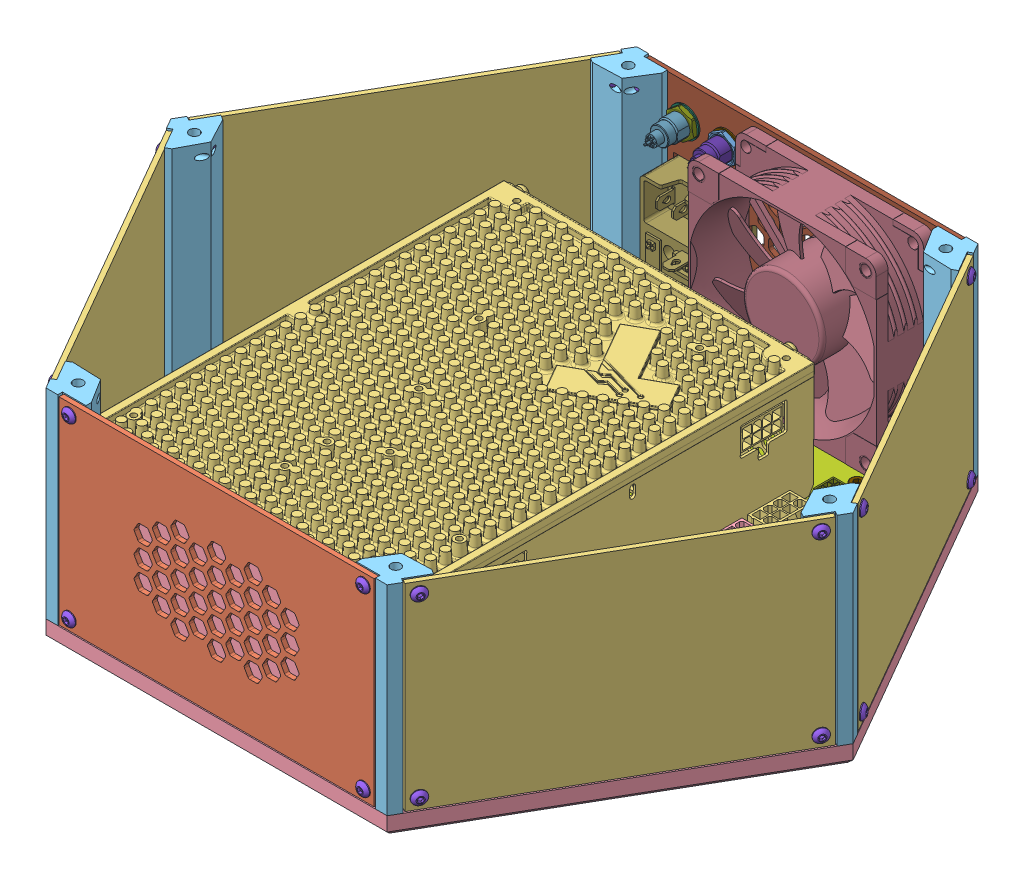
SolidWorks assembly base_assembly, configuration Default. Lengths in mm. (continued)
Components (placement in the parent): (continued)
- zaphod-controller-1: zaphod-controller [Default] at (56 14 107.9) x (0 0 -1) z (0 1 0) size (199.92 69.34 18.57) (continued)
  - SOT95P240X110-3L16-18: SOT95P240X110-3L16 [Default] at (114 -66.9 1.65) size (2.91 3.01 1.23) (continued)
    - COMPOUND_6-1: COMPOUND_6 [Default] at origin size (2.91 3.01 1.23)
  - SOT95P240X110-3L16-19: SOT95P240X110-3L16 [Default] at (114 -61.2 1.65) size (2.91 3.01 1.23)
    - COMPOUND_6-1: COMPOUND_6 [Default] at origin size (2.91 3.01 1.23)
  - SOT95P240X110-3L16-20: SOT95P240X110-3L16 [Default] at (141.5 -23.1 1.65) x (0 -1 0) z (0 0 1) size (2.91 3.01 1.23)
    - COMPOUND_6-1: COMPOUND_6 [Default] at origin size (2.91 3.01 1.23)
  - SOT95P240X110-3L16-21: SOT95P240X110-3L16 [Default] at (122.4 -45.4 1.65) x (-1 0 0) z (0 0 1) size (2.91 3.01 1.23)
    - COMPOUND_6-1: COMPOUND_6 [Default] at origin size (2.91 3.01 1.23)
  - RESC1608X50-9: RESC1608X50 [Default] at (169.2907 -2.1731 -0.05) x (1 0 0) z (0 0 -1) size (1.6 0.8 0.5)
    - COMPOUND_5-1: COMPOUND_5 [Default] at origin size (1.6 0.8 0.5)
  - RESC1608X50-10: RESC1608X50 [Default] at (169.2907 -4.1731 -0.05) x (-1 0 0) z (0 0 -1) size (1.6 0.8 0.5)
    - COMPOUND_5-1: COMPOUND_5 [Default] at origin size (1.6 0.8 0.5)
  - RESC1608X50-11: RESC1608X50 [Default] at (169.2907 -6.1731 -0.05) x (1 0 0) z (0 0 -1) size (1.6 0.8 0.5)
    - COMPOUND_5-1: COMPOUND_5 [Default] at origin size (1.6 0.8 0.5)
  - RESC1608X50-12: RESC1608X50 [Default] at (103 -51 1.65) x (0 -1 0) z (0 0 1) size (1.6 0.8 0.5)
    - COMPOUND_5-1: COMPOUND_5 [Default] at origin size (1.6 0.8 0.5)
  - RESC1608X50-13: RESC1608X50 [Default] at (32.7 -21 1.65) x (-1 0 0) z (0 0 1) size (1.6 0.8 0.5)
    - COMPOUND_5-1: COMPOUND_5 [Default] at origin size (1.6 0.8 0.5)
  - RESC1608X50-14: RESC1608X50 [Default] at (29.2 -19.75 1.65) size (1.6 0.8 0.5)
    - COMPOUND_5-1: COMPOUND_5 [Default] at origin size (1.6 0.8 0.5)
  - RESC1608X50-15: RESC1608X50 [Default] at (96.275 -42.75 1.65) x (-1 0 0) z (0 0 1) size (1.6 0.8 0.5)
    - COMPOUND_5-1: COMPOUND_5 [Default] at origin size (1.6 0.8 0.5)
  - RESC1608X50-16: RESC1608X50 [Default] at (106.5 -51 1.65) x (0 1 0) z (0 0 1) size (1.6 0.8 0.5)
    - COMPOUND_5-1: COMPOUND_5 [Default] at origin size (1.6 0.8 0.5)
  - RESC1608X50-17: RESC1608X50 [Default] at (106.5 -47.5 1.65) x (0 1 0) z (0 0 1) size (1.6 0.8 0.5)
    - COMPOUND_5-1: COMPOUND_5 [Default] at origin size (1.6 0.8 0.5)
  - RESC1608X50-18: RESC1608X50 [Default] at (32.7 -18 1.65) x (-1 0 0) z (0 0 1) size (1.6 0.8 0.5)
    - COMPOUND_5-1: COMPOUND_5 [Default] at origin size (1.6 0.8 0.5)
  - RESC1608X50-19: RESC1608X50 [Default] at (29.2 -18 1.65) x (-1 0 0) z (0 0 1) size (1.6 0.8 0.5)
    - COMPOUND_5-1: COMPOUND_5 [Default] at origin size (1.6 0.8 0.5)
  - RESC1608X50-20: RESC1608X50 [Default] at (32.7 -27 1.65) x (-1 0 0) z (0 0 1) size (1.6 0.8 0.5)
    - COMPOUND_5-1: COMPOUND_5 [Default] at origin size (1.6 0.8 0.5)
  - RESC1608X50-21: RESC1608X50 [Default] at (29.45 -28.75 1.65) x (-1 0 0) z (0 0 1) size (1.6 0.8 0.5)
    - COMPOUND_5-1: COMPOUND_5 [Default] at origin size (1.6 0.8 0.5)
  - RESC1608X50-22: RESC1608X50 [Default] at (32.7 -28.75 1.65) x (-1 0 0) z (0 0 1) size (1.6 0.8 0.5)
    - COMPOUND_5-1: COMPOUND_5 [Default] at origin size (1.6 0.8 0.5)
  - RESC1608X50-23: RESC1608X50 [Default] at (41.1 -23.3 -0.05) x (-1 0 0) z (0 0 -1) size (1.6 0.8 0.5)
    - COMPOUND_5-1: COMPOUND_5 [Default] at origin size (1.6 0.8 0.5)
  - RESC1608X50-24: RESC1608X50 [Default] at (53.05 -17.05 1.65) x (0 -1 0) z (0 0 1) size (1.6 0.8 0.5)
    - COMPOUND_5-1: COMPOUND_5 [Default] at origin size (1.6 0.8 0.5)
  - RESC1608X50-25: RESC1608X50 [Default] at (49.8 -19.05 1.65) x (-1 0 0) z (0 0 1) size (1.6 0.8 0.5)
    - COMPOUND_5-1: COMPOUND_5 [Default] at origin size (1.6 0.8 0.5)
  - RESC1608X50-26: RESC1608X50 [Default] at (87 -51 1.65) x (0 -1 0) z (0 0 1) size (1.6 0.8 0.5)
    - COMPOUND_5-1: COMPOUND_5 [Default] at origin size (1.6 0.8 0.5)
  - RESC1608X50-27: RESC1608X50 [Default] at (55.2 -20.25 -0.05) x (0 -1 0) z (0 0 -1) size (1.6 0.8 0.5)
    - COMPOUND_5-1: COMPOUND_5 [Default] at origin size (1.6 0.8 0.5)
  - RESC1608X50-28: RESC1608X50 [Default] at (49.8 -23.05 1.65) x (-1 0 0) z (0 0 1) size (1.6 0.8 0.5)
    - COMPOUND_5-1: COMPOUND_5 [Default] at origin size (1.6 0.8 0.5)
  - RESC1608X50-29: RESC1608X50 [Default] at (49.8 -21.3 1.65) x (-1 0 0) z (0 0 1) size (1.6 0.8 0.5)
    - COMPOUND_5-1: COMPOUND_5 [Default] at origin size (1.6 0.8 0.5)
  - RESC1608X50-30: RESC1608X50 [Default] at (49.8 -24.8 1.65) x (-1 0 0) z (0 0 1) size (1.6 0.8 0.5)
    - COMPOUND_5-1: COMPOUND_5 [Default] at origin size (1.6 0.8 0.5)
  - RESC3216X140-1: RESC3216X140 [Default] at (66.9 -26.05 1.65) x (-1 0 0) z (0 0 1) size (3.2 1.6 1.4)
    - COMPOUND_13-1: COMPOUND_13 [Default] at origin size (3.2 1.6 1.4)
  - RESC1608X50-31: RESC1608X50 [Default] at (80.275 -42.75 1.65) x (-1 0 0) z (0 0 1) size (1.6 0.8 0.5)
    - COMPOUND_5-1: COMPOUND_5 [Default] at origin size (1.6 0.8 0.5)
  - RESC1608X50-32: RESC1608X50 [Default] at (90.5 -51 1.65) x (0 1 0) z (0 0 1) size (1.6 0.8 0.5)
    - COMPOUND_5-1: COMPOUND_5 [Default] at origin size (1.6 0.8 0.5)
  - RESC1608X50-33: RESC1608X50 [Default] at (90.5 -47.525 1.65) x (0 1 0) z (0 0 1) size (1.6 0.8 0.5)
    - COMPOUND_5-1: COMPOUND_5 [Default] at origin size (1.6 0.8 0.5)
  - RESC1608X50-34: RESC1608X50 [Default] at (118.4 -64 1.65) x (-1 0 0) z (0 0 1) size (1.6 0.8 0.5)
    - COMPOUND_5-1: COMPOUND_5 [Default] at origin size (1.6 0.8 0.5)
  - R_Array_Concave_4x060-1: R_Array_Concave_4x060 [Default] at (130.8 -40.6 1.65) x (0 -1 0) z (-1 0 0) size (3.2 0.65 1.6)
    - SOLID_22-1: SOLID_22 [Default] at origin size (3.2 0.65 1.6)
  - RESC1608X50-35: RESC1608X50 [Default] at (143.3978 -41.5245 1.65) x (-0.866025 -0.5 0) z (0 0 1) size (1.6 0.8 0.5)
    - COMPOUND_5-1: COMPOUND_5 [Default] at origin size (1.6 0.8 0.5)
  - RESC1608X50-36: RESC1608X50 [Default] at (142.4978 -39.9657 1.65) x (-0.866025 -0.5 0) z (0 0 1) size (1.6 0.8 0.5)
    - COMPOUND_5-1: COMPOUND_5 [Default] at origin size (1.6 0.8 0.5)
  - RESC1608X50-37: RESC1608X50 [Default] at (123.6 -36.6 -0.05) x (1 0 0) z (0 0 -1) size (1.6 0.8 0.5)
    - COMPOUND_5-1: COMPOUND_5 [Default] at origin size (1.6 0.8 0.5)
  - RESC1608X50-38: RESC1608X50 [Default] at (179.1 -22.4 1.65) x (0 1 0) z (0 0 1) size (1.6 0.8 0.5)
    - COMPOUND_5-1: COMPOUND_5 [Default] at origin size (1.6 0.8 0.5)
  - RESC1608X50-39: RESC1608X50 [Default] at (175.1 -22.5 1.65) x (0 -1 0) z (0 0 1) size (1.6 0.8 0.5)
    - COMPOUND_5-1: COMPOUND_5 [Default] at origin size (1.6 0.8 0.5)
  - R_Array_Concave_4x060-2: R_Array_Concave_4x060 [Default] at (114.4 -18.6 1.65) x (-1 0 0) z (0 1 0) size (3.2 0.65 1.6)
    - SOLID_22-1: SOLID_22 [Default] at origin size (3.2 0.65 1.6)
  - RESC1608X50-40: RESC1608X50 [Default] at (30 -12.8 -0.05) x (-1 0 0) z (0 0 -1) size (1.6 0.8 0.5)
    - COMPOUND_5-1: COMPOUND_5 [Default] at origin size (1.6 0.8 0.5)
  - RESC1608X50-41: RESC1608X50 [Default] at (64.9267 -12.8 -0.05) x (-1 0 0) z (0 0 -1) size (1.6 0.8 0.5)
    - COMPOUND_5-1: COMPOUND_5 [Default] at origin size (1.6 0.8 0.5)
  - RESC1608X50-42: RESC1608X50 [Default] at (99.9 -12.8 -0.05) x (-1 0 0) z (0 0 -1) size (1.6 0.8 0.5)
    - COMPOUND_5-1: COMPOUND_5 [Default] at origin size (1.6 0.8 0.5)
  - RESC1608X50-43: RESC1608X50 [Default] at (134.8 -12.8 -0.05) x (-1 0 0) z (0 0 -1) size (1.6 0.8 0.5)
    - COMPOUND_5-1: COMPOUND_5 [Default] at origin size (1.6 0.8 0.5)
  - RESC1608X50-44: RESC1608X50 [Default] at (46 -18.2 -0.05) x (-1 0 0) z (0 0 -1) size (1.6 0.8 0.5)
    - COMPOUND_5-1: COMPOUND_5 [Default] at origin size (1.6 0.8 0.5)
  - RESC1608X50-45: RESC1608X50 [Default] at (81 -18.4 -0.05) x (-1 0 0) z (0 0 -1) size (1.6 0.8 0.5)
    - COMPOUND_5-1: COMPOUND_5 [Default] at origin size (1.6 0.8 0.5)
  - RESC1608X50-46: RESC1608X50 [Default] at (115.9727 -18.4 -0.05) x (-1 0 0) z (0 0 -1) size (1.6 0.8 0.5)
    - COMPOUND_5-1: COMPOUND_5 [Default] at origin size (1.6 0.8 0.5)
  - RESC1608X50-47: RESC1608X50 [Default] at (151 -18.4 -0.05) x (-1 0 0) z (0 0 -1) size (1.6 0.8 0.5)
    - COMPOUND_5-1: COMPOUND_5 [Default] at origin size (1.6 0.8 0.5)
  - RESC1608X50-48: RESC1608X50 [Default] at (44.9727 -15.623 -0.05) x (0 -1 0) z (0 0 -1) size (1.6 0.8 0.5)
    - COMPOUND_5-1: COMPOUND_5 [Default] at origin size (1.6 0.8 0.5)
  - RESC1608X50-49: RESC1608X50 [Default] at (80 -15.6 -0.05) x (0 -1 0) z (0 0 -1) size (1.6 0.8 0.5)
    - COMPOUND_5-1: COMPOUND_5 [Default] at origin size (1.6 0.8 0.5)
  - RESC1608X50-50: RESC1608X50 [Default] at (114.9727 -15.598 -0.05) x (0 -1 0) z (0 0 -1) size (1.6 0.8 0.5)
    - COMPOUND_5-1: COMPOUND_5 [Default] at origin size (1.6 0.8 0.5)
  - RESC1608X50-51: RESC1608X50 [Default] at (150.0554 -15.6 -0.05) x (0 -1 0) z (0 0 -1) size (1.6 0.8 0.5)
    - COMPOUND_5-1: COMPOUND_5 [Default] at origin size (1.6 0.8 0.5)
  - R_Array_Concave_4x060-3: R_Array_Concave_4x060 [Default] at (182.7 -15.1 -0.05) x (0 -1 0) z (1 0 0) size (3.2 0.65 1.6)
    - SOLID_22-1: SOLID_22 [Default] at origin size (3.2 0.65 1.6)
  - RESC1608X50-52: RESC1608X50 [Default] at (182.7 -27.1 -0.05) x (-1 0 0) z (0 0 -1) size (1.6 0.8 0.5)
    - COMPOUND_5-1: COMPOUND_5 [Default] at origin size (1.6 0.8 0.5)
  - RESC1608X50-53: RESC1608X50 [Default] at (182.7 -25.4 -0.05) x (-1 0 0) z (0 0 -1) size (1.6 0.8 0.5)
    - COMPOUND_5-1: COMPOUND_5 [Default] at origin size (1.6 0.8 0.5)
  - RESC1608X50-54: RESC1608X50 [Default] at (182.7442 -23.7 -0.05) x (-1 0 0) z (0 0 -1) size (1.6 0.8 0.5)
    - COMPOUND_5-1: COMPOUND_5 [Default] at origin size (1.6 0.8 0.5)
  - RESC1608X50-55: RESC1608X50 [Default] at (182.7442 -22 -0.05) x (-1 0 0) z (0 0 -1) size (1.6 0.8 0.5)
    - COMPOUND_5-1: COMPOUND_5 [Default] at origin size (1.6 0.8 0.5)
  - RESC1608X50-56: RESC1608X50 [Default] at (119.4 -66.9 1.65) x (0 1 0) z (0 0 1) size (1.6 0.8 0.5)
    - COMPOUND_5-1: COMPOUND_5 [Default] at origin size (1.6 0.8 0.5)
  - RESC1608X50-57: RESC1608X50 [Default] at (117.5 -66.9 1.65) x (0 1 0) z (0 0 1) size (1.6 0.8 0.5)
    - COMPOUND_5-1: COMPOUND_5 [Default] at origin size (1.6 0.8 0.5)
  - RESC1608X50-58: RESC1608X50 [Default] at (114.1 -64 1.65) size (1.6 0.8 0.5)
    - COMPOUND_5-1: COMPOUND_5 [Default] at origin size (1.6 0.8 0.5)
  - R_Array_Concave_4x060-4: R_Array_Concave_4x060 [Default] at (130.8 -31.6 1.65) x (0 1 0) z (1 0 0) size (3.2 0.65 1.6)
    - SOLID_22-1: SOLID_22 [Default] at origin size (3.2 0.65 1.6)
  - RESC1608X50-59: RESC1608X50 [Default] at (138.6 -23.9 1.65) x (0 -1 0) z (0 0 1) size (1.6 0.8 0.5)
    - COMPOUND_5-1: COMPOUND_5 [Default] at origin size (1.6 0.8 0.5)
  - RESC1608X50-60: RESC1608X50 [Default] at (145.4685 -24.8 1.65) size (1.6 0.8 0.5)
    - COMPOUND_5-1: COMPOUND_5 [Default] at origin size (1.6 0.8 0.5)
  - RESC1608X50-61: RESC1608X50 [Default] at (117.2 -45.3548 1.65) x (0 -1 0) z (0 0 1) size (1.6 0.8 0.5)
    - COMPOUND_5-1: COMPOUND_5 [Default] at origin size (1.6 0.8 0.5)
  - RESC1608X50-62: RESC1608X50 [Default] at (119.2 -45.3548 1.65) x (0 -1 0) z (0 0 1) size (1.6 0.8 0.5)
    - COMPOUND_5-1: COMPOUND_5 [Default] at origin size (1.6 0.8 0.5)
  - RESC1608X50-63: RESC1608X50 [Default] at (145.4685 -26.4833 1.65) x (-1 0 0) z (0 0 1) size (1.6 0.8 0.5)
    - COMPOUND_5-1: COMPOUND_5 [Default] at origin size (1.6 0.8 0.5)
  - RESC1608X50-64: RESC1608X50 [Default] at (145.5 -23.1 1.65) size (1.6 0.8 0.5)
    - COMPOUND_5-1: COMPOUND_5 [Default] at origin size (1.6 0.8 0.5)
  - RESC1608X50-65: RESC1608X50 [Default] at (145.4685 -28.2 1.65) x (-1 0 0) z (0 0 1) size (1.6 0.8 0.5)
    - COMPOUND_5-1: COMPOUND_5 [Default] at origin size (1.6 0.8 0.5)
  - B3U-1000P-1: B3U-1000P [Default] at (122 -66.2 1.65) x (0 1 0) z (1 0 0) size (4 1.6 2.5)
    - SOLID_23-1: SOLID_23 [Default] at origin size (4 1.6 2.5)
  - B3U-1000P-2: B3U-1000P [Default] at (151.4 -49.3 1.65) x (0.5 -0.866025 0) z (-0.866025 -0.5 0) size (4 1.6 2.5)
    - SOLID_23-1: SOLID_23 [Default] at origin size (4 1.6 2.5)
  - B3U-1000P-3: B3U-1000P [Default] at (146.8 -51.8 1.65) x (0.5 -0.866025 0) z (-0.866025 -0.5 0) size (4 1.6 2.5)
    - SOLID_23-1: SOLID_23 [Default] at origin size (4 1.6 2.5)
  - KEYSTONE_5115_BROWN-1: KEYSTONE_5115_BROWN [Default] at (52.8 -42.8 1.65) x (0 1 0) z (0 0 1) size (2.54 2.54 7.62)
    - COMPOUND_14-1: COMPOUND_14 [Default] at origin size (2.54 2.54 7.62)
  - KEYSTONE_5004_YELLOW-1: KEYSTONE_5004_YELLOW [Default] at (73.4 -54.4 1.65) x (0 1 0) z (0 0 1) size (2.54 2.54 7.62)
    - COMPOUND_15-1: COMPOUND_15 [Default] at origin size (2.54 2.54 7.62)
  - KEYSTONE_5000_RED-1: KEYSTONE_5000_RED [Default] at (83.4 -60.8 1.65) x (0 1 0) z (0 0 1) size (2.54 2.54 7.62)
    - COMPOUND_16-1: COMPOUND_16 [Default] at origin size (2.54 2.54 7.62)
  - KEYSTONE_5003_ORANGE-1: KEYSTONE_5003_ORANGE [Default] at (95.4 -64.2 1.65) x (0 1 0) z (0 0 1) size (2.54 2.54 7.62)
    - COMPOUND_17-1: COMPOUND_17 [Default] at origin size (2.54 2.54 7.62)
  - KEYSTONE_5001_BLACK-1: KEYSTONE_5001_BLACK [Default] at (62 -48.4 1.65) x (0 1 0) z (0 0 1) size (2.54 2.54 7.62)
    - COMPOUND_18-1: COMPOUND_18 [Default] at origin size (2.54 2.54 7.62)
  - RESC1608X50-66: RESC1608X50 [Default] at (142 -35.6 1.65) x (0 -1 0) z (0 0 1) size (1.6 0.8 0.5)
    - COMPOUND_5-1: COMPOUND_5 [Default] at origin size (1.6 0.8 0.5)
  - QFN50P400X300X100-13T170X330-1: QFN50P400X300X100-13T170X330 [Default] at (101.25 -46.5 1.65) x (0 -1 0) z (-1 0 0) size (4 1.08 3.08)
    - SOLID_24-1: SOLID_24 [Default] at origin size (4 1.08 3.08)
  - SOP20P65_720X780X200L75X30L-1: SOP20P65_720X780X200L75X30L [Default] at (41.1 -19.3 1.65) x (0 -1 0) z (-1 0 0) size (7.2 1.9 7.8)
    - COMPOUND_19-1: COMPOUND_19 [Default] at origin size (7.2 1.9 7.8)
  - QFN50P400X300X100-13T170X330-2: QFN50P400X300X100-13T170X330 [Default] at (85.25 -46.5 1.65) x (0 -1 0) z (-1 0 0) size (4 1.08 3.08)
    - SOLID_24-1: SOLID_24 [Default] at origin size (4 1.08 3.08)
  - ACS-EX-12-1: ACS-EX-12 [Default] at (33.2 -11.9 6.55) x (-1 0 0) z (0 0 -1) size (3 3 0.73)
    - SOLID_25-1: SOLID_25 [Default] at origin size (3 3 0.73)
  - ACS-EX-12-2: ACS-EX-12 [Default] at (68.1767 -11.9216 6.55) x (-1 0 0) z (0 0 -1) size (3 3 0.73)
    - SOLID_25-1: SOLID_25 [Default] at origin size (3 3 0.73)
  - ACS-EX-12-3: ACS-EX-12 [Default] at (103.15 -11.95 6.55) x (-1 0 0) z (0 0 -1) size (3 3 0.73)
    - SOLID_25-1: SOLID_25 [Default] at origin size (3 3 0.73)
  - ACS-EX-12-4: ACS-EX-12 [Default] at (138.15 -11.95 6.55) x (-1 0 0) z (0 0 -1) size (3 3 0.73)
    - SOLID_25-1: SOLID_25 [Default] at origin size (3 3 0.73)
  - SOIC127P1030X265-18L87-1: SOIC127P1030X265-18L87 [Default] at (90.298 -28.0273 -0.05) x (0 1 0) z (0 0 -1) size (11.35 10.17 2)
    - COMPOUND_20-1: COMPOUND_20 [Default] at origin size (11.35 10.17 2)
  - SOIC127P1030X265-18L87-2: SOIC127P1030X265-18L87 [Default] at (140.602 -28.0727 -0.05) x (0 -1 0) z (0 0 -1) size (11.35 10.17 2)
    - COMPOUND_20-1: COMPOUND_20 [Default] at origin size (11.35 10.17 2)
  - CNCTECH_3220-10-0300-1: CNCTECH_3220-10-0300 [Default] at (131.2 -61.5 1.65) x (0.866025 0.5 0) z (0.5 -0.866025 0) size (12.65 5.6 5.5)
    - COMPOUND_21-1: COMPOUND_21 [Default] at origin size (12.65 5.6 5.5)
  - XTALDFN200X120X60-2-1: XTALDFN200X120X60-2 [Default] at (125.6 -35.6 1.65) x (0 1 0) z (1 0 0) size (2.01 0.61 1.19)
    - SOLID_26-1: SOLID_26 [Default] at origin size (2.01 0.61 1.19)
  - CAPAE1350X1350D1490DD450L470-1: CAPAE1350X1350D1490DD450L470 [Default] at (44.7 -34 1.65) x (0.5 0.866025 0) z (0.866025 -0.5 0) size (13.7 14 15)
    - COMPOUND_22-1: COMPOUND_22 [Default] at origin size (13.7 14 15)
  - RESC1608X50-67: RESC1608X50 [Default] at (53.8 -27.2 -0.05) x (1 0 0) z (0 0 -1) size (1.6 0.8 0.5)
    - COMPOUND_5-1: COMPOUND_5 [Default] at origin size (1.6 0.8 0.5)
  - COMPOUND_23-1: COMPOUND_23 [Default] at origin size (199.92 69.34 1.6)
- hexagon socket head cap screw_as-1: hexagon socket head cap screw_as [AS 1420 - M3 x 5-N] at (120 18.6 0) x (0 -1 0) z (0 0 1) size (8 5.5 5.5)
- hexagon socket head cap screw_as-2: hexagon socket head cap screw_as [AS 1420 - M3 x 5-N] at (60 18.6 103.923) x (0 -1 0) z (0 0 1) size (8 5.5 5.5)
- hexagon socket head cap screw_as-3: hexagon socket head cap screw_as [AS 1420 - M3 x 5-N] at (60.5 19.2333 -86.2) x (0 -1 0) z (0 0 1) size (8 5.5 5.5)
Mates (geometry in assembly coordinates):
- Concentric1871: concentric aligned: cylinder of side_cover_full-1 through (77.5 13 -116.9134) axis (0.866025 0 -0.5) radius 1.7; cylinder of socket button head cap screw_am-2 through (78.9289 13 -117.7384) axis (0.866025 0 -0.5) radius 1.5
- Coincident4871: coincident anti-aligned: plane of side_cover_full-1 through (75.25 92.5 -120.8105) normal (0.866025 0 -0.5); plane of socket button head cap screw_am-2 through (77.7065 14.442 -116.5558) normal (-0.866025 0 0.5)
- Concentric1881: concentric aligned: cylinder of side_cover_full-1 through (140 13 -8.6603) axis (0.866025 0 -0.5) radius 1.7; cylinder of socket button head cap screw_am-3 through (141.4289 13 -9.4853) axis (0.866025 0 -0.5) radius 1.5
- Coincident4881: coincident anti-aligned: plane of side_cover_full-1 through (75.25 92.5 -120.8105) normal (0.866025 0 -0.5); plane of socket button head cap screw_am-3 through (140.2065 14.442 -8.3026) normal (-0.866025 0 0.5)
- Concentric1891: concentric aligned: cylinder of side_cover_full-1 through (140 88 -8.6603) axis (0.866025 0 -0.5) radius 1.7; cylinder of socket button head cap screw_am-4 through (141.4289 88 -9.4853) axis (0.866025 0 -0.5) radius 1.5
- Coincident4891: coincident anti-aligned: plane of side_cover_full-1 through (75.25 92.5 -120.8105) normal (0.866025 0 -0.5); plane of socket button head cap screw_am-4 through (140.6838 88.616 -7.4758) normal (-0.866025 0 0.5)
- Concentric1901: concentric aligned: cylinder of side_cover_full-1 through (77.5 88 -116.9134) axis (0.866025 0 -0.5) radius 1.7; cylinder of socket button head cap screw_am-5 through (78.9289 88 -117.7384) axis (0.866025 0 -0.5) radius 1.5
- Coincident4901: coincident anti-aligned: plane of side_cover_full-1 through (75.25 92.5 -120.8105) normal (0.866025 0 -0.5); plane of socket button head cap screw_am-5 through (77.7065 89.442 -116.5558) normal (-0.866025 0 0.5)
- Concentric2021: concentric aligned: cylinder of electronics_panel-1/side_cover_fan-1 through (62.5 88 -125.5737) axis (0 0 -1) radius 1.7; cylinder of socket button head cap screw_am-23 through (62.5 88 -127.2237) axis (0 0 -1) radius 1.5
- Coincident5191: coincident anti-aligned: plane of electronics_panel-1/side_cover_fan-1 through (67 8.5 -125.5737) normal (0 0 -1); plane of socket button head cap screw_am-23 through (63.1515 89.3511 -125.5737) normal (0 0 1)
- Concentric2031: concentric aligned: cylinder of electronics_panel-1/side_cover_fan-1 through (-62.5 88 -125.5737) axis (0 0 -1) radius 1.7; cylinder of socket button head cap screw_am-24 through (-62.5 88 -127.2237) axis (0 0 -1) radius 1.5
- Coincident5201: coincident anti-aligned: plane of electronics_panel-1/side_cover_fan-1 through (67 8.5 -125.5737) normal (0 0 -1); plane of socket button head cap screw_am-24 through (-61.8485 89.3511 -125.5737) normal (0 0 1)
- Concentric2041: concentric aligned: cylinder of electronics_panel-1/side_cover_fan-1 through (-62.5 13 -125.5737) axis (0 0 -1) radius 1.7; cylinder of socket button head cap screw_am-25 through (-62.5 13 -127.2237) axis (0 0 -1) radius 1.5
- Coincident5211: coincident anti-aligned: plane of electronics_panel-1/side_cover_fan-1 through (67 8.5 -125.5737) normal (0 0 -1); plane of socket button head cap screw_am-25 through (-61.8485 14.3511 -125.5737) normal (0 0 1)
- Concentric2051: concentric aligned: cylinder of electronics_panel-1/side_cover_fan-1 through (62.5 13 -125.5737) axis (0 0 -1) radius 1.7; cylinder of socket button head cap screw_am-26 through (62.5 13 -127.2237) axis (0 0 -1) radius 1.5
- Coincident5221: coincident anti-aligned: plane of electronics_panel-1/side_cover_fan-1 through (67 8.5 -125.5737) normal (0 0 -1); plane of socket button head cap screw_am-26 through (63.1515 14.3511 -125.5737) normal (0 0 1)
- Concentric20601: concentric aligned: cylinder of side_cover_vent-1 through (-62.5 88 125.5737) axis (0 0 1) radius 1.7; cylinder of socket button head cap screw_am-27 through (-62.5 88 127.2237) axis (0 0 1) radius 1.5
- Coincident52551: coincident anti-aligned: plane of side_cover_vent-1 through (-67 8.5 125.5737) normal (0 0 1); plane of socket button head cap screw_am-27 through (-61.4966 89.1149 125.5737) normal (0 0 -1)
- Concentric20611: concentric aligned: cylinder of side_cover_vent-1 through (62.5 88 125.5737) axis (0 0 1) radius 1.7; cylinder of socket button head cap screw_am-28 through (62.5 88 127.2237) axis (0 0 1) radius 1.5
- Coincident52561: coincident anti-aligned: plane of side_cover_vent-1 through (-67 8.5 125.5737) normal (0 0 1); plane of socket button head cap screw_am-28 through (63.5034 89.1149 125.5737) normal (0 0 -1)
- Concentric20621: concentric aligned: cylinder of side_cover_vent-1 through (62.5 13 125.5737) axis (0 0 1) radius 1.7; cylinder of socket button head cap screw_am-29 through (62.5 13 127.2237) axis (0 0 1) radius 1.5
- Coincident52571: coincident anti-aligned: plane of side_cover_vent-1 through (-67 8.5 125.5737) normal (0 0 1); plane of socket button head cap screw_am-29 through (63.5034 14.1149 125.5737) normal (0 0 -1)
- Concentric20631: concentric aligned: cylinder of side_cover_vent-1 through (-62.5 13 125.5737) axis (0 0 1) radius 1.7; cylinder of socket button head cap screw_am-30 through (-62.5 13 127.2237) axis (0 0 1) radius 1.5
- Coincident52581: coincident anti-aligned: plane of side_cover_vent-1 through (-67 8.5 125.5737) normal (0 0 1); plane of socket button head cap screw_am-30 through (-61.4966 14.1149 125.5737) normal (0 0 -1)
- Width13: width anti-aligned: plane of demci_filter_0887-1 through (-48.5 15 121.1737) normal (0 -1 0); plane of demci_filter_0887-1 through (-48.5 86 121.1737) normal (0 1 0); plane of side_cover_vent-1 through (-67 92.5 125.5737) normal (0 1 0); plane of side_cover_vent-1 through (-67 8.5 125.5737) normal (0 -1 0)
- Width14: width anti-aligned: plane of demci_filter_0887-1 through (48.5 15 121.1737) normal (1 0 0); plane of demci_filter_0887-1 through (-48.5 15 121.1737) normal (-1 0 0); plane of side_cover_vent-1 through (-67 8.5 125.5737) normal (-1 0 0); plane of side_cover_vent-1 through (67 8.5 125.5737) normal (1 0 0)
- Coincident5259: coincident anti-aligned: plane of side_cover_vent-1 through (-67 8.5 123.5737) normal (0 0 -1); plane of demci_filter_0887-1 through (0 50.5 123.5737) normal (0 0 1)
- Coincident52593: coincident anti-aligned: plane of frame_bottom_assembly-1/bottom_plate_detail-1 through (0 8 0) normal (0 1 0); plane of psu_assembly-1/psu_mount-1 through (-81.5 8 97.5737) normal (0 -1 0)
- Concentric20634: concentric anti-aligned: cylinder of frame_bottom_assembly-1/bottom_plate_detail-1 through (-50 0 88.5737) axis (0 -1 0) radius 2.75; cylinder of psu_assembly-1/psu_mount-1 through (-50 12 88.5737) axis (0 1 0) radius 2.1
- Concentric20635: concentric anti-aligned: cylinder of frame_bottom_assembly-1/bottom_plate_detail-1 through (-70 0 88.5737) axis (0 -1 0) radius 2.75; cylinder of psu_assembly-1/psu_mount-1 through (-70 12 88.5737) axis (0 1 0) radius 2.1
- Coincident52594: coincident anti-aligned: plane of frame_bottom_assembly-1/frame_pillar-1 through (57.5 8 -123.5737) normal (0 0 -1); plane of electronics_panel-1/side_cover_fan-1 through (67 8.5 -123.5737) normal (0 0 1)
- Width15: width aligned: plane of frame_bottom_assembly-1/frame_pillar-1 through (67.5 8 -123.5737) normal (-1 0 0); plane of frame_bottom_assembly-1/frame_pillar-3 through (-67.5 8 -123.5737) normal (1 0 0); plane of electronics_panel-1/side_cover_fan-1 through (-67 8.5 -125.5737) normal (-1 0 0); plane of electronics_panel-1/side_cover_fan-1 through (67 8.5 -125.5737) normal (1 0 0)
- Concentric20636: concentric aligned: cylinder of frame_bottom_assembly-1/frame_pillar-1 through (62.5 13 -123.5737) axis (0 0 -1) radius 1.25; cylinder of socket button head cap screw_am-26 through (62.5 13 -127.2237) axis (0 0 -1) radius 1.5
- Coincident52595: coincident anti-aligned: plane of frame_bottom_assembly-1/frame_pillar-7 through (135.7679 8 -11.9904) normal (0.866025 0 -0.5); plane of side_cover_full-1 through (73.5179 92.5 -119.8105) normal (-0.866025 0 0.5)
- Width16: width anti-aligned: plane of frame_bottom_assembly-1/frame_pillar-7 through (140.7679 8 -3.3301) normal (-0.5 0 -0.866025); plane of frame_bottom_assembly-1/frame_pillar-1 through (73.2679 8 -120.2436) normal (0.5 0 0.866025); plane of side_cover_full-1 through (142.25 92.5 -4.7631) normal (0.5 0 0.866025); plane of side_cover_full-1 through (75.25 92.5 -120.8105) normal (-0.5 0 -0.866025)
- Concentric20637: concentric aligned: cylinder of frame_bottom_assembly-1/frame_pillar-7 through (138.2679 13 -7.6603) axis (0.866025 0 -0.5) radius 1.25; cylinder of socket button head cap screw_am-3 through (141.4289 13 -9.4853) axis (0.866025 0 -0.5) radius 1.5
- Width17: width anti-aligned: plane of side_cover_vent-1 through (67 8.5 125.5737) normal (1 0 0); plane of side_cover_vent-1 through (-67 8.5 125.5737) normal (-1 0 0); plane of frame_bottom_assembly-1/frame_pillar-6 through (67.5 8 123.5737) normal (-1 0 0); plane of frame_bottom_assembly-1/frame_pillar-5 through (-67.5 8 123.5737) normal (1 0 0)
- Coincident52597: coincident anti-aligned: plane of frame_bottom_assembly-1/frame_pillar-6 through (57.5 8 123.5737) normal (0 0 1); plane of side_cover_vent-1 through (-67 8.5 123.5737) normal (0 0 -1)
- Concentric20638: concentric aligned: cylinder of frame_bottom_assembly-1/frame_pillar-6 through (62.5 13 123.5737) axis (0 0 1) radius 1.25; cylinder of socket button head cap screw_am-29 through (62.5 13 127.2237) axis (0 0 1) radius 1.5
- Coincident52598: coincident anti-aligned: plane of frame_bottom_assembly-1/bottom_plate_detail-1 through (0 0 0) normal (0 -1 0); plane of assembly through (0 0 0) normal (0 1 0)
- Symmetric2: symmetric aligned: plane of frame_bottom_assembly-1/bottom_plate_detail-1 through (-72.5 0 -125.5737) normal (0 0 -1); plane of frame_bottom_assembly-1/bottom_plate_detail-1 through (72.5 0 125.5737) normal (0 0 1); plane of assembly through (0 0 0) normal (0 0 1)
- Symmetric1: symmetric: moEndPointRef_w of frame_bottom_assembly-1/bottom_plate_detail-1; moEndPointRef_w of frame_bottom_assembly-1/bottom_plate_detail-1; plane of assembly
- Concentric20639: concentric aligned: cylinder of frame_bottom_assembly-1/M3_standoff-2 through (120 14 0) axis (0 1 0) radius 1.25; cylinder of zaphod-controller-1/COMPOUND_23-1 through (120 13.2 0) axis (0 1 0) radius 1.6
- Concentric20640: concentric aligned: cylinder of frame_bottom_assembly-1/M3_standoff-3 through (60 14 103.923) axis (0 1 0) radius 1.25; cylinder of zaphod-controller-1/COMPOUND_23-1 through (60 13.2 103.923) axis (0 1 0) radius 1.6
- Parallel1: parallel aligned: cylinder of frame_bottom_assembly-1/M3_standoff-1 through (60 14 -86.077) axis (0 1 0) radius 1.25; cylinder of zaphod-controller-1/COMPOUND_23-1 through (60.5 13.2 -86.2) axis (0 1 0) radius 1.6
- Coincident52599: coincident anti-aligned: plane of frame_bottom_assembly-1/M3_standoff-1 through (60 14 -86.077) normal (0 1 0); plane of zaphod-controller-1/COMPOUND_23-1 through (56 14 -88) normal (0 -1 0)
- Concentric206421: concentric aligned: cylinder of zaphod-controller-1/COMPOUND_23-1 through (120 13.2 0) axis (0 1 0) radius 1.6; cylinder of hexagon socket head cap screw_as-1 through (120 15.6 0) axis (0 1 0) radius 2.75
- Coincident526001: coincident anti-aligned: plane of zaphod-controller-1/COMPOUND_23-1 through (56 15.6 -88) normal (0 1 0); plane of hexagon socket head cap screw_as-1 through (120 15.6 0) normal (0 -1 0)
- Concentric20643: concentric aligned: cylinder of zaphod-controller-1/COMPOUND_23-1 through (60 13.2 103.923) axis (0 1 0) radius 1.6; cylinder of hexagon socket head cap screw_as-2 through (60 15.6 103.923) axis (0 1 0) radius 2.75
- Coincident52601: coincident anti-aligned: plane of zaphod-controller-1/COMPOUND_23-1 through (56 15.6 -88) normal (0 1 0); plane of hexagon socket head cap screw_as-2 through (60 15.6 103.923) normal (0 -1 0)
- Concentric20644: concentric aligned: cylinder of zaphod-controller-1/COMPOUND_23-1 through (60.5 13.2 -86.2) axis (0 1 0) radius 1.6; cylinder of hexagon socket head cap screw_as-3 through (60.5 16.2333 -86.2) axis (0 1 0) radius 2.75
